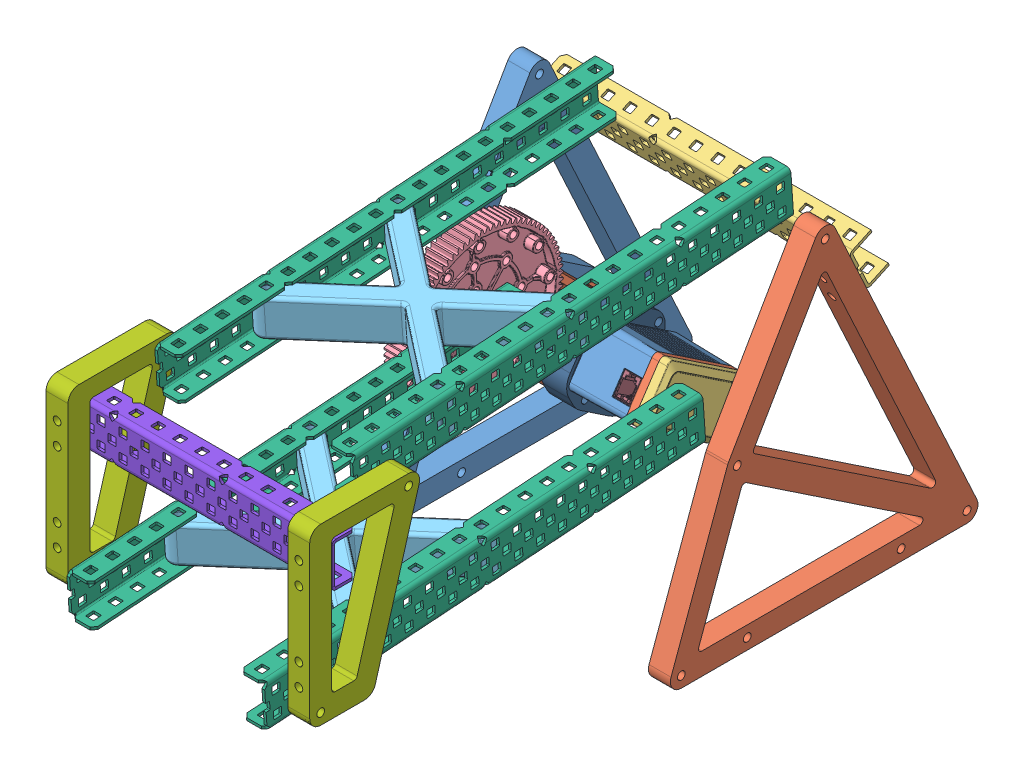
SolidWorks assembly RearArmAssembly, configuration Default. Lengths in mm.
Overall size (177.8 196.8 382.98).
43 component instances, 23 part files, 28 mates.
Components (placement in the parent):
- ArmMount-1: ArmMount [Default] at (3.0815 119.4615 170.9285) size (12.7 189.78 177.8)
- ArmMount(mirror)-1: ArmMount(mirror) [Default] at (168.1815 119.4615 170.9285) size (12.7 189.78 177.8)
- 1x2x1x14 Aluminum C-Channel-1: 1x2x1x14 Aluminum C-Channel [Default] at (225.3315 181.5036 101.1108) x (1 0 0) z (0 -0.420336 0.907368) size (177.8 25.41 13.97)
- RearArm_BottomBar-1: RearArm_BottomBar [Default] at (222.7102 54.1717 183.8088) x (0 -0.069828 0.997559) z (-1 0 0) size (286.79 90.98 127)
  - 84T High Strength Gear (276-3438)-1: 84T High Strength Gear (276-3438) [Default] at (-17.4079 64.2311 194.2288) size (90.98 90.98 12.7)
  - ArmXBrace-1: ArmXBrace [Default] at (128.6421 53.1059 130.7288) x (0 0 1) z (-1 0 0) size (111.86 22.25 88.94)
  - 1x2x1x20 Aluminum C-Channel-1: 1x2x1x20 Aluminum C-Channel [Default] at (192.1421 64.2311 187.8788) size (254 25.41 13.97)
  - 1x2x1x20 Aluminum C-Channel-2: 1x2x1x20 Aluminum C-Channel [Default] at (192.1421 64.2311 73.5788) x (1 0 0) z (0 0 -1) size (254 25.41 13.97)
- RearArm_TopBar-1: RearArm_TopBar [Default] at (12.5514 278.2747 177.0234) x (0 -0.069828 0.997559) z (1 0 0) size (254 25.4 114.31)
  - ArmXBrace-1: ArmXBrace [Default] at (94.2395 63.4998 79.4301) x (0 0 1) z (-1 0 0) size (111.86 22.25 88.94)
  - 1x2x1x20 Aluminum C-Channel-1: 1x2x1x20 Aluminum C-Channel [Default] at (157.7395 74.625 136.5801) size (254 25.41 13.97)
  - 1x2x1x20 Aluminum C-Channel-2: 1x2x1x20 Aluminum C-Channel [Default] at (157.7395 74.625 22.2801) x (1 0 0) z (0 0 -1) size (254 25.41 13.97)
- ArmEndAssembly-1: ArmEndAssembly [Default] at (208.3285 70.3449 488.0787) x (-1 0 0) z (0 0 -1) size (152.48 100.69 63.5)
  - ArmEnd-1: ArmEnd [Default] at (40.147 33.1539 89.1082) size (12.7 100.69 63.5)
  - ArmEnd-2: ArmEnd [Default] at (179.847 33.1539 89.1082) size (12.7 100.69 63.5)
  - 1x2x1x12 Aluminum C-Channel-1: 1x2x1x12 Aluminum C-Channel [Default] at (262.3169 103.0039 95.4582) x (1 0 0) z (0 0 -1) size (152.4 25.41 13.97)
- 0.5in 0.375in OD Nylon Spacer-1: 0.5in 0.375in OD Nylon Spacer [Default] at (22.1315 87.6603 123.4437) x (0 1 0) z (0 0 1) size (9.53 12.7 9.53)
- ArmMotorMount-1: ArmMotorMount [Default] at (41.1815 87.6603 123.4437) x (0 0.830879 -0.556452) z (1 0 0) size (48.1 53.1 15)
- 1.00_ Standoff (275-1016)-1: 1.00_ Standoff (275-1016) [Default] at (28.4815 71.832 134.0442) x (0 -1 0) z (0 0 1) size (7.34 25.4 7.34)
- 1.00_ Standoff (275-1016)-2: 1.00_ Standoff (275-1016) [Default] at (28.4815 103.4885 112.8433) x (0 -1 0) z (0 0 1) size (7.34 25.4 7.34)
- 1.00_ Standoff (275-1016)-3: 1.00_ Standoff (275-1016) [Default] at (28.4815 57.6981 112.9398) x (0 -1 0) z (0 0 1) size (7.34 25.4 7.34)
- 1.00_ Standoff (275-1016)-4: 1.00_ Standoff (275-1016) [Default] at (28.4815 89.3546 91.739) x (0 -1 0) z (0 0 1) size (7.34 25.4 7.34)
- V5 Smart Motor (276-4840) no cap-1: V5 Smart Motor (276-4840) no cap [Default] at (73.3815 80.5933 112.8916) x (0 0.556452 0.830879) z (-1 0 0) size (59.01 35.33 59.91)
  - V5 Smart Motor (276-4840).step-1: V5 Smart Motor (276-4840).step [Default] at origin size (59.01 35.33 59.91)
    - 276-4840-900 Rev6_Instruction.step-1: 276-4840-900 Rev6_Instruction.step [Default] at (-14.3 0 -17.2) size (52.79 15.94 38.15)
      - 276-4840-901 Rev6.step-1: 276-4840-901 Rev6.step [Default] at (10.75 -10.05 17.8) x (-1 0 0) z (0 0 1) size (49.9 1.6 38.15)
      - 276-4840-902 Rev2.step-1: 276-4840-902 Rev2.step [Default] at (31.25 -9.25 6.2) x (0 0 -1) z (0 -1 0) size (10.35 11.39 15.94)
      - 276-4840-022 Rev4.step-1: 276-4840-022 Rev4.step [Default] at (31.25 -9.25 6.2) x (0 0 -1) z (1 0 0) size (10.26 9.1 5.51)
    - 276-4840-110 Rev10_Instruction.step-1: 276-4840-110 Rev10_Instruction.step [Default] at (12.7 0 14.7) size (35.33 35.33 31.1)
      - 276-4840-061 Rev7_Ring_Gear_Fixed01 .6 Rev3.step-1: 276-4840-061 Rev7_Ring_Gear_Fixed01 .6 Rev3.step [Default] at origin size (28.79 28.39 24.6)
      - 276-4840-018 Rev6.step-1: 276-4840-018 Rev6.step [Default] at (0 0 6.7) x (-0.483174 0.875524 0) z (0 0 1) size (26 26 12.3)
      - 276-4840-059 Rev2.step-1: 276-4840-059 Rev2.step [Default] at (0 0 10.3) size (28.4 28.4 8.5)
      - 276-4840-062 Rev1.step-1: 276-4840-062 Rev1.step [Default] at (-12.1353 8.8168 12.3) x (0.956835 -0.290632 0) z (-0.290632 -0.956835 0) size (3.2 6.56 3.2)
      - 276-4840-062 Rev1.step-2: 276-4840-062 Rev1.step [Default] at (12.1353 8.8168 12.3) x (0.978427 0.206591 0) z (0.206591 -0.978427 0) size (3.2 6.56 3.2)
      - 276-4840-062 Rev1.step-3: 276-4840-062 Rev1.step [Default] at (-12.1353 -8.8168 12.3) x (0.72563 0.688086 0) z (0.688086 -0.72563 0) size (3.2 6.56 3.2)
    - 276-4840-001 Rev38.step-1: 276-4840-001 Rev38.step [Default] at origin size (57.3 33 46.9)
    - 276-4840-005 Rev27.step-1: 276-4840-005 Rev27.step [Default] at (0 0 -17.95) size (56.17 31.87 12.9)
    - 276-4840-004 Rev16.step-1: 276-4840-004 Rev16.step [Default] at (0 0 -19.2) size (56.01 31.71 9.21)
    - 276-4840-009 Rev3.step-1: 276-4840-009 Rev3.step [Default] at (25.45 13.5 15.7) x (0.19987 -0.979823 0) z (-0.979823 -0.19987 0) size (3.4 41.31 4.34)
    - 276-4840-009 Rev3.step-2: 276-4840-009 Rev3.step [Default] at (-25.45 -13.5 15.7) x (-0.998855 0.047836 0) z (0.047836 0.998855 0) size (3.4 41.31 4.34)
    - 276-4840-009 Rev3.step-3: 276-4840-009 Rev3.step [Default] at (25.45 -13.5 15.7) x (-0.975374 0.220559 0) z (0.220559 0.975374 0) size (3.4 41.31 4.34)
    - 276-4840-009 Rev3.step-4: 276-4840-009 Rev3.step [Default] at (-25.45 13.5 15.7) x (-0.922256 0.38658 0) z (0.38658 0.922256 0) size (3.4 41.31 4.34)
    - 276-4840-025 Rev19.step-1: 276-4840-025 Rev19.step [Default] at (12.7 0 -22.63) x (-0.993315 0.115437 0) z (0 0 1) size (14.82 14.83 35.18)
Mates (geometry in assembly coordinates):
- Concentric1: concentric aligned: cylinder of ArmMount-1 through (15.7815 30.5615 203.2855) axis (-1 0 0) radius 2.25; cylinder of ArmMount(mirror)-1 through (180.8815 30.5615 203.2855) axis (-1 0 0) radius 2.25
- Concentric2: concentric aligned: cylinder of ArmMount-1 through (15.7815 30.5615 165.1855) axis (-1 0 0) radius 2.25; cylinder of ArmMount(mirror)-1 through (180.8815 30.5615 165.1855) axis (-1 0 0) radius 2.25
- Coincident2: coincident anti-aligned: plane of ArmMount-1 through (15.7815 24.2115 28.2456) normal (0 0.420336 -0.907368); plane of 1x2x1x14 Aluminum C-Channel-1 through (3.5815 161.6138 91.8969) normal (0 -0.420336 0.907368)
- Concentric5: concentric anti-aligned: cylinder of ArmMount-1 through (9.4315 118.0828 253.1226) axis (0 0.420336 -0.907368) radius 2.25; circle of 1x2x1x14 Aluminum C-Channel-1
- Concentric6: concentric anti-aligned: cylinder of ArmMount(mirror)-1 through (174.5315 118.0828 253.1226) axis (0 0.420336 -0.907368) radius 2.25; circle of 1x2x1x14 Aluminum C-Channel-1
- Concentric11: concentric aligned: cylinder of ArmMount-1 through (15.7815 119.4615 170.9285) axis (-1 0 0) radius 2.25; circle of RearArm_BottomBar-1/1x2x1x20 Aluminum C-Channel-1
- Distance4: distance = 19.05 mm anti-aligned: plane of RearArm_BottomBar-1/1x2x1x20 Aluminum C-Channel-1 through (34.8315 98.4466 157.2276) normal (-1 0 0); plane of ArmMount-1 through (15.7815 119.4615 170.9285) normal (1 0 0)
- Distance5: distance = 19.05 mm anti-aligned: plane of RearArm_TopBar-1/1x2x1x20 Aluminum C-Channel-2 through (34.8315 186.4348 106.4276) normal (-1 0 0); plane of ArmMount-1 through (15.7815 119.4615 170.9285) normal (1 0 0)
- Concentric14: concentric anti-aligned: circle of RearArm_BottomBar-1/1x2x1x20 Aluminum C-Channel-1; cylinder of ArmEndAssembly-1/ArmEnd-2 through (15.7815 103.4989 398.9705) axis (1 0 0) radius 2.25
- Distance6: distance = 6.35 mm anti-aligned: plane of RearArm_BottomBar-1/1x2x1x20 Aluminum C-Channel-1 through (34.8315 98.4466 157.2276) normal (-1 0 0); plane of ArmEndAssembly-1/ArmEnd-2 through (28.4815 103.4989 398.9705) normal (1 0 0)
- Concentric15: concentric aligned: cylinder of ArmMount-1 through (15.7815 207.4497 120.1285) axis (-1 0 0) radius 2.25; circle of RearArm_TopBar-1/1x2x1x20 Aluminum C-Channel-2
- Concentric16: concentric anti-aligned: circle of RearArm_TopBar-1/1x2x1x20 Aluminum C-Channel-2; cylinder of ArmEndAssembly-1/ArmEnd-2 through (15.7815 191.487 348.1705) axis (1 0 0) radius 2.25
- Coincident9: coincident anti-aligned: plane of ArmMount-1 through (9.4315 87.6603 123.4437) normal (1 0 0); plane of 0.5in 0.375in OD Nylon Spacer-1 through (9.4315 87.6603 123.4437) normal (-1 0 0)
- Concentric17: concentric aligned: cylinder of ArmMount-1 through (9.4315 87.6603 123.4437) axis (1 0 0) radius 4.7625; cylinder of 0.5in 0.375in OD Nylon Spacer-1 through (9.4315 87.6603 123.4437) axis (1 0 0) radius 4.7625
- Concentric20: concentric anti-aligned: cylinder of ArmMount-1 through (15.7815 89.3546 91.739) axis (-1 0 0) radius 2.25; cylinder of 1.00_ Standoff (275-1016)-4 through (15.7815 89.3546 91.739) axis (1 0 0) radius 2.0955
- Concentric21: concentric anti-aligned: cylinder of ArmMount-1 through (15.7815 57.6981 112.9398) axis (-1 0 0) radius 2.25; cylinder of 1.00_ Standoff (275-1016)-3 through (15.7815 57.6981 112.9398) axis (1 0 0) radius 2.0955
- Concentric22: concentric anti-aligned: cylinder of ArmMount-1 through (15.7815 103.4885 112.8433) axis (-1 0 0) radius 2.25; cylinder of 1.00_ Standoff (275-1016)-2 through (15.7815 103.4885 112.8433) axis (1 0 0) radius 2.0955
- Concentric23: concentric anti-aligned: cylinder of ArmMount-1 through (15.7815 71.832 134.0442) axis (-1 0 0) radius 2.25; cylinder of 1.00_ Standoff (275-1016)-1 through (15.7815 71.832 134.0442) axis (1 0 0) radius 2.0955
- Coincident11: coincident anti-aligned: plane of ArmMount-1 through (15.7815 119.4615 170.9285) normal (1 0 0); plane of 1.00_ Standoff (275-1016)-1 through (15.7815 73.6651 130.8692) normal (-1 0 0)
- Coincident12: coincident anti-aligned: plane of ArmMount-1 through (15.7815 119.4615 170.9285) normal (1 0 0); plane of 1.00_ Standoff (275-1016)-3 through (15.7815 59.5312 109.7648) normal (-1 0 0)
- Coincident13: coincident anti-aligned: plane of ArmMount-1 through (15.7815 119.4615 170.9285) normal (1 0 0); plane of 1.00_ Standoff (275-1016)-4 through (15.7815 91.1877 88.564) normal (-1 0 0)
- Coincident14: coincident anti-aligned: plane of ArmMount-1 through (15.7815 119.4615 170.9285) normal (1 0 0); plane of 1.00_ Standoff (275-1016)-2 through (15.7815 105.3216 109.6683) normal (-1 0 0)
- Coincident15: coincident anti-aligned: plane of ArmMotorMount-1 through (41.1815 87.6603 123.4437) normal (-1 0 0); plane of 1.00_ Standoff (275-1016)-4 through (41.1815 91.1877 88.564) normal (1 0 0)
- Concentric24: concentric anti-aligned: cylinder of ArmMotorMount-1 through (56.1815 103.4885 112.8433) axis (-1 0 0) radius 2.25; cylinder of 1.00_ Standoff (275-1016)-2 through (15.7815 103.4885 112.8433) axis (1 0 0) radius 2.0955
- Concentric28: concentric aligned: cylinder of ArmMotorMount-1 through (56.1815 73.5264 102.3394) axis (-1 0 0) radius 4.3; cone of V5 Smart Motor (276-4840) no cap-1/V5 Smart Motor (276-4840).step-1/276-4840-001 Rev38.step-1 through (43.6815 73.5264 102.3394) axis (-1 0 0)
- Coincident16: coincident anti-aligned: plane of ArmMotorMount-1 through (56.1815 87.6603 123.4437) normal (1 0 0); plane of V5 Smart Motor (276-4840) no cap-1/V5 Smart Motor (276-4840).step-1/276-4840-001 Rev38.step-1 through (56.1815 77.3725 84.8998) normal (-1 0 0)
- Parallel2: parallel aligned: line of ArmMotorMount-1 through (56.1815 104.7161 122.8531) axis (0 -0.556452 -0.830879); line of V5 Smart Motor (276-4840) no cap-1/V5 Smart Motor (276-4840).step-1/276-4840-001 Rev38.step-1 through (57.1815 108.242 124.5236) axis (0 -0.556452 -0.830879)
- Parallel3: parallel aligned: plane of ArmMount-1 through (15.7815 98.3572 185.0624) normal (0 -0.830879 0.556452); plane of ArmMotorMount-1 through (56.1815 67.6776 136.8264) normal (0 -0.830879 0.556452)
